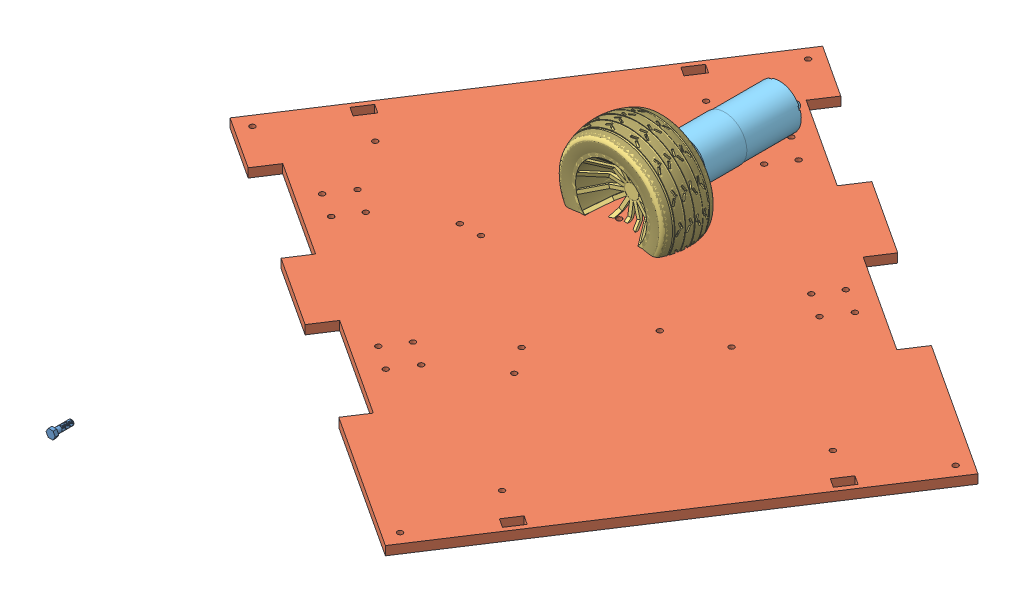
SolidWorks assembly Assem1, configuration Default. Lengths in mm.
Overall size (392.81 64.99 409.11).
6 component instances, 6 part files, 4 mates.
Components (placement in the parent):
- l2Mbolt-1: l2Mbolt [Default] at (-5.6801 7.2132 13.9259) size (5.19 4.62 12)
- down chasse-1: down chasse [Default] at (77.9205 2.8689 -211.6791) x (-0.837169 0 -0.546944) z (-0.546944 0 0.837169) size (300 5 259)
- Part1^Assem11-1: Part1^Assem11 [Default] at origin (virtual)
- l2Mtire-1: l2Mtire [Défaut] at (48.3587 16.237 -259.2631) x (0 0 -1) z (1 0 0) size (29.78 64.99 64.99)
- Mirrornew motor holder-1: Mirrornew motor holder [Default] at (35.8587 -0.763 -283.8088) size (25 31.5 33)
- Mirrordc motor-1: Mirrordc motor [Default] at (48.3587 16.237 -339.6088) x (-0.923728 -0.383049 0) z (0 0 -1) size (25 25 72.3)
Mates (geometry in assembly coordinates):
- Coincident8: coincident anti-aligned: circle of Mirrornew motor holder-1; circle of Mirrordc motor-1
- Coincident9: coincident: circle of l2Mtire-1; circle of Mirrordc motor-1
- Coincident16: coincident: circle of down chasse-1; circle of Mirrornew motor holder-1
- Coincident22: coincident: circle of down chasse-1; circle of Mirrornew motor holder-1
